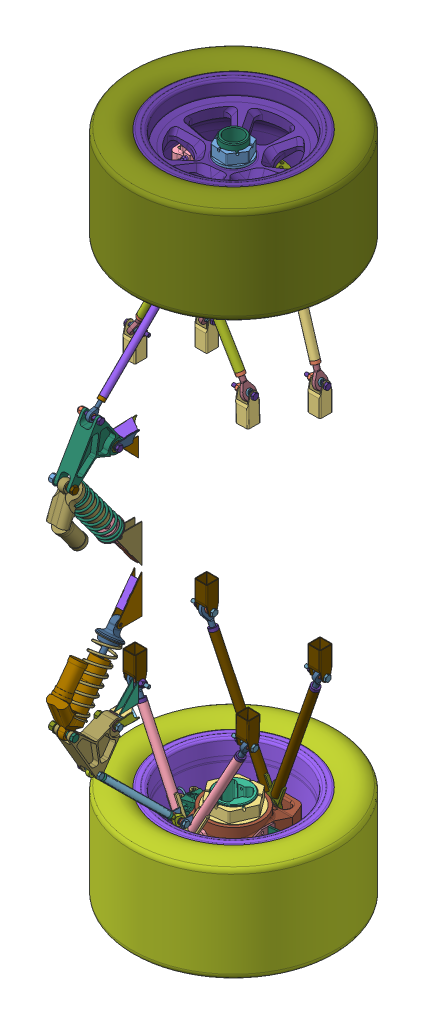
SolidWorks assembly UN-A1001-AA-Rear Unsprung Assembly, configuration Default. Lengths in mm.
Overall size (998.86 1363.58 600.2).
282 component instances, 120 part files, 8 mates.
Components (placement in the parent):
- SP-A0200-AH-Rear Axle Assembly-1: SP-A0200-AH-Rear Axle Assembly [Default] at origin size (935.94 549.59 593.34)
  - SP-AA-Rear Lower A-Arm^SP-A0200-AH-Rear Axle Assembly-1: SP-AA-Rear Lower A-Arm^SP-A0200-AH-Rear Axle Assembly [Default] at (0 -0.399 0.6588) x (1 0 0) z (0 0.002866 0.999996) size (222.76 290.57 36.42) (virtual)
    - SP-Lower Apex Rear-1: SP-Lower Apex Rear [Default] at (-792.4265 549.6462 121.5417) x (-0.932505 -0.360479 0.022123) z (0 -0.061256 -0.998122) size (54.94 63.8 9.53)
    - MirrorFS-MALE ROD END UNF-3A, 0.3125x24-0.25D (XAM-4)1-1: MirrorFS-MALE ROD END UNF-3A, 0.3125x24-0.25D (XAM-4)1 [Default] at (-906.7265 255.0788 139.6197) x (0.932505 -0.360479 0.022123) z (-0.361157 -0.930754 0.057121)
    - MirrorFS-MALE ROD END UNF-3A, 0.3125x24-0.25D (XAM-4)1-2: MirrorFS-MALE ROD END UNF-3A, 0.3125x24-0.25D (XAM-4)1 [Default] at (-678.1265 255.0788 139.6197) x (0.932505 0.360479 -0.022123) z (0.361157 -0.930754 0.057121)
    - SP-10003-AB-Threaded Insert-1: SP-10003-AB-Threaded Insert [A-Arm] at (-890.6731 296.4508 137.0806) x (0.932505 -0.360479 0.022123) z (-0.361157 -0.930754 0.057121) size (15.88 15.88 15.88)
    - SP-10003-AB-Threaded Insert-2: SP-10003-AB-Threaded Insert [A-Arm] at (-694.18 296.4508 137.0806) x (0.932505 0.360479 -0.022123) z (0.361157 -0.930754 0.057121) size (15.88 15.88 15.88)
    - SP-Rear Lower A-Arm Tube-1: SP-Rear Lower A-Arm Tube [Default] at (-838.6322 430.5677 128.8497) x (-0.361157 -0.930754 0.057121) z (0 -0.061256 -0.998122) size (257.84 15.88 15.88)
    - SP-Rear Lower A-Arm Tube-2: SP-Rear Lower A-Arm Tube [Default] at (-746.2209 430.5677 128.8497) x (0.361157 -0.930754 0.057121) z (0 0.061256 0.998122) size (257.84 15.88 15.88)
    - FS-HIGH MISALIGN SPHERICAL BEARING, 0.375-0.906D (3072-6G)-1: FS-HIGH MISALIGN SPHERICAL BEARING, 0.375-0.906D (3072-6G) [Default] at (-792.4265 549.6462 121.5417) x (-0.932505 0.360479 -0.022123) z (-0.361157 -0.930754 0.057121) size (26.46 21.71 26.13)
      - Race^FS-HIGH MISALIGN SPHERICAL BEARING, 0.375-0.906D (3072-6G)-1: Race^FS-HIGH MISALIGN SPHERICAL BEARING, 0.375-0.906D (3072-6G) [Default] at origin size (23.01 8.76 23.01) (virtual)
      - Ball^FS-HIGH MISALIGN SPHERICAL BEARING, 0.375-0.906D (3072-6G)-1: Ball^FS-HIGH MISALIGN SPHERICAL BEARING, 0.375-0.906D (3072-6G) [Default] x (0.359576 -0.008176 0.93308) z (-0.932238 -0.046516 0.358844) size (19.84 20.65 19.84) (virtual)
  - SP-AA-Rear Upper A-Arm^SP-A0200-AH-Rear Axle Assembly-1: SP-AA-Rear Upper A-Arm^SP-A0200-AH-Rear Axle Assembly [Default] at (-38.1 -1.9308 1.9372) x (1 0 0) z (0 0.00685 0.999977) size (216 215.55 29.43) (virtual)
    - SP-Upper Apex Rear-1: SP-Upper Apex Rear [Default] at (-755.8405 523.8827 293.8505) x (0.884705 -0.465567 -0.023329) z (0 -0.050046 0.998747) size (76.45 83.12 9.53)
    - MirrorFS-MALE ROD END UNF-3A, 0.3125x24-0.25D (XAM-4)1-1: MirrorFS-MALE ROD END UNF-3A, 0.3125x24-0.25D (XAM-4)1 [Default] at (-870.1405 307.2255 282.9942) x (0.884705 -0.465567 -0.023329) z (-0.466151 -0.883596 -0.044276)
    - MirrorFS-MALE ROD END UNF-3A, 0.3125x24-0.25D (XAM-4)1-2: MirrorFS-MALE ROD END UNF-3A, 0.3125x24-0.25D (XAM-4)1 [Default] at (-641.5405 307.2255 282.9942) x (0.884705 0.465567 0.023329) z (0.466151 -0.883596 -0.044276)
    - SP-10003-AB-Threaded Insert-1: SP-10003-AB-Threaded Insert [A-Arm] at (-849.4201 346.5014 284.9623) x (0.884705 -0.465567 -0.023329) z (-0.466151 -0.883596 -0.044276) size (15.88 15.88 15.88)
    - SP-10003-AB-Threaded Insert-2: SP-10003-AB-Threaded Insert [A-Arm] at (-662.261 346.5014 284.9623) x (0.884705 0.465567 0.023329) z (0.466151 -0.883596 -0.044276) size (15.88 15.88 15.88)
    - SP-Rear Upper A-Arm Tube-1: SP-Rear Upper A-Arm Tube [Default] at (-812.9905 415.5541 288.4224) x (0.466151 0.883596 0.044276) z (0.884705 -0.465567 -0.023329) size (186.28 15.88 15.88)
    - SP-Rear Upper A-Arm Tube-2: SP-Rear Upper A-Arm Tube [Default] at (-698.6905 415.5541 288.4224) x (-0.466151 0.883596 0.044276) z (0.884705 0.465567 0.023329) size (186.28 15.88 15.88)
    - FS-HIGH MISALIGN SPHERICAL BEARING, 0.375-0.906D (3072-6G)-1: FS-HIGH MISALIGN SPHERICAL BEARING, 0.375-0.906D (3072-6G) [Default] at (-755.8405 523.8827 293.8505) x (0.884705 -0.465567 -0.023329) z (-0.466151 -0.883596 -0.044276) size (26.46 21.71 26.13)
      - Race^FS-HIGH MISALIGN SPHERICAL BEARING, 0.375-0.906D (3072-6G)-1: Race^FS-HIGH MISALIGN SPHERICAL BEARING, 0.375-0.906D (3072-6G) [Default] at origin size (23.01 8.76 23.01) (virtual)
      - Ball^FS-HIGH MISALIGN SPHERICAL BEARING, 0.375-0.906D (3072-6G)-1: Ball^FS-HIGH MISALIGN SPHERICAL BEARING, 0.375-0.906D (3072-6G) [Default] x (0.359576 -0.008176 0.93308) z (-0.932238 -0.046516 0.358844) size (19.84 20.65 19.84) (virtual)
  - Assem8^SP-A0200-AH-Rear Axle Assembly-1: Assem8^SP-A0200-AH-Rear Axle Assembly [Default] at (-1592.9214 814.7933 712.2762) x (-0.999891 -0.01037 0.010464) z (0.012143 -0.982316 0.186836) size (17.98 166.51 230.13) (virtual)
    - Part2^Assem8_SP-A0200-AH-Rear Axle Assembly-1: Part2^Assem8_SP-A0200-AH-Rear Axle Assembly [Default] at origin size (15.39 113.92 157.78) (virtual)
    - SP-10003-AC-Threaded Insert-2: SP-10003-AC-Threaded Insert [AM-4 Rod End Thread] at (-799.064 427.6015 294.0449) x (-0.999891 -0.008342 0.012143) z (-0.014733 0.566176 -0.824153) size (12.7 12.7 15.88)
    - SP-10003-AC-Threaded Insert-3: SP-10003-AC-Threaded Insert [AM-4 Rod End Thread] at (-796.6527 334.9355 428.9338) x (-0.999891 -0.008342 0.012143) z (0.014733 -0.566176 0.824153) size (12.7 12.7 15.88)
    - FS-MALE ROD END UNF-3A, 0.25x28-0.25D (AM-4)-1: FS-MALE ROD END UNF-3A, 0.25x28-0.25D (AM-4) [Default] at (-796.0446 311.5665 462.9507) x (0 -0.824242 -0.566238) z (-0.014733 0.566176 -0.824153) size (19.32 14.06 49.44)
      - Body^FS-MALE ROD END UNF-3A, 0.25x28-0.25D (AM-4)-2: Body^FS-MALE ROD END UNF-3A, 0.25x28-0.25D (AM-4) [Default] at origin size (19.32 7.2 49.44) (virtual)
      - Ball^FS-MALE ROD END UNF-3A, 0.25x28-0.25D (AM-4)-2: Ball^FS-MALE ROD END UNF-3A, 0.25x28-0.25D (AM-4) [Default] x (0.09633 0.218783 0.971007) z (-0.984027 0.167661 0.059845) size (12.7 9.53 12.7) (virtual)
    - FS-MALE ROD END UNF-3A, 0.25x28-0.25D (AM-4)-2: FS-MALE ROD END UNF-3A, 0.25x28-0.25D (AM-4) [Default] at (-799.6721 450.9704 260.028) x (0 -0.824242 -0.566238) z (0.014733 -0.566176 0.824153) size (19.32 14.06 49.44)
      - Body^FS-MALE ROD END UNF-3A, 0.25x28-0.25D (AM-4)-2: Body^FS-MALE ROD END UNF-3A, 0.25x28-0.25D (AM-4) [Default] at origin size (19.32 7.2 49.44) (virtual)
      - Ball^FS-MALE ROD END UNF-3A, 0.25x28-0.25D (AM-4)-2: Ball^FS-MALE ROD END UNF-3A, 0.25x28-0.25D (AM-4) [Default] x (0.09633 0.218783 0.971007) z (-0.984027 0.167661 0.059845) size (12.7 9.53 12.7) (virtual)
  - SP-A0105-AC-Ohlin TTX25 MKII, 200mm-1: SP-A0105-AC-Ohlin TTX25 MKII, 200mm [Default] at (-793.9406 216.4917 537.8809) x (-1 0 0) z (0 0.803503 0.5953) size (48.39 85.02 197.6)
    - Shock Body^SP-A0105-AC-Ohlin TTX25 MKII, 200mm-1: Shock Body^SP-A0105-AC-Ohlin TTX25 MKII, 200mm [Default] at origin size (40.76 80 131.7) (virtual)
    - Head^SP-A0105-AC-Ohlin TTX25 MKII, 200mm-1: Head^SP-A0105-AC-Ohlin TTX25 MKII, 200mm [Default] at (0 0 -174.6) size (46 46 119) (virtual)
    - Ball^SP-A0105-AC-Ohlin TTX25 MKII, 200mm-1: Ball^SP-A0105-AC-Ohlin TTX25 MKII, 200mm [Default] at (0 0 -174.6) x (-0.011681 0.107343 0.994153) z (0.993776 0.111394 -0.000351) size (15 15 8) (virtual)
    - Ball^SP-A0105-AC-Ohlin TTX25 MKII, 200mm-2: Ball^SP-A0105-AC-Ohlin TTX25 MKII, 200mm [Default] x (0.079523 -0.862756 -0.499328) z (0.965926 -0.057074 0.252448) size (15 15 8) (virtual)
    - SP-#####-AB-Spring-1: SP-#####-AB-Spring [Default] at (0 0 -151.1) size (48.39 49.05 127.97)
  - FS-BALL BEARING, 0.25ID-0.75OD (60355K702)-1: FS-BALL BEARING, 0.25ID-0.75OD (60355K702) [Default] at (-784.8125 243.84 446.6415) x (0 -0.287121 0.957894) z (-1 0 0) size (19.05 19.05 7.14)
  - FS-BALL BEARING, 0.25ID-0.75OD (60355K702)-2: FS-BALL BEARING, 0.25ID-0.75OD (60355K702) [Default] at (-803.0688 243.84 446.6415) x (0 0.287121 -0.957894) z (1 0 0) size (19.05 19.05 7.14)
  - FS-CADMIUM PLATED C3 HEX, 0.25x28-1.65-0.469 (AN4-13A)-2: FS-CADMIUM PLATED C3 HEX, 0.25x28-1.65-0.469 (AN4-13A) [Default] at (-796.8362 310.0391 484.3789) x (-1 0 0) z (0 0.868755 0.495242) size (46.28 12.9 11.18)
  - FS-ZINC YELLOW CHROMATE C10.9 HX, M8x1.25-40-22 (95327A569)-1: FS-ZINC YELLOW CHROMATE C10.9 HX, M8x1.25-40-22 (95327A569) [Default] at (-795.4156 216.4917 537.8809) x (-1 0 0) z (0 -0.287121 0.957894) size (45.3 15.01 13)
  - FS-NYLOC FLHX C8, M8x1.25-11.1 (92461A400)-1: FS-NYLOC FLHX C8, M8x1.25-11.1 (92461A400) [Default] at (-820.9156 216.4917 537.8809) x (0 0.868058 -0.496463) z (-1 0 0) size (17.9 17.9 11.1)
  - FS-NYLOC G8 HX, 0.25x28-0.3125 (90630A145)-1: FS-NYLOC G8 HX, 0.25x28-0.3125 (90630A145) [Default] at (-809.8156 310.0391 484.3789) x (0 0.868058 -0.496463) z (0 0.496463 0.868058) size (11.11 7.94 12.83)
  - SP-C30066-AA-A-Arm Tab Box-1: SP-C30066-AA-A-Arm Tab Box [Default] at (-680.9758 289.7175 282.8202) x (-0.029021 0.999579 0) z (0 0 -1) size (60.32 25.4 25.4)
  - SP-C30066-AA-A-Arm Tab Box-2: SP-C30066-AA-A-Arm Tab Box [Default] at (-908.2405 289.7636 282.8202) x (0 1 0) z (0 0 -1) size (60.32 25.4 25.4)
  - SP-C30066-AA-A-Arm Tab Box-3: SP-C30066-AA-A-Arm Tab Box [Default] at (-678.1265 237.6164 139.5469) x (0 1 0) z (0 0 1) size (60.32 25.4 25.4)
  - SP-C30066-AA-A-Arm Tab Box-4: SP-C30066-AA-A-Arm Tab Box [Default] at (-906.7265 237.6164 139.5469) x (0 1 0) z (0 0 1) size (60.32 25.4 25.4)
  - MirrorSP-30063-AB-Pushrod Tab-1: MirrorSP-30063-AB-Pushrod Tab [Default] at (-782.0343 483.2134 293.6084) x (1 0 0) z (0 0.043203 -0.999066) size (1.59 15.88 23.81)
  - MirrorSP-30063-AB-Pushrod Tab-2: MirrorSP-30063-AB-Pushrod Tab [Default] at (-805.8468 483.2134 293.6084) x (-1 0 0) z (0 0.043203 -0.999066) size (1.59 15.88 23.81)
  - FS-NYLOC FLHX C8, M8x1.25-11.1 (92461A400)-2: FS-NYLOC FLHX C8, M8x1.25-11.1 (92461A400) [Default] at (-820.9156 243.84 446.6415) x (0 0 -1) z (-1 0 0) size (17.9 17.9 11.1)
  - FS-CADMIUM PLATED C3 HEX, 0.25x28-1.65-0.469 (AN4-13A)-3: FS-CADMIUM PLATED C3 HEX, 0.25x28-1.65-0.469 (AN4-13A) [Default] at (-796.8362 243.84 446.6415) x (-1 0 0) z (0 0.287121 -0.957894) size (46.28 12.9 11.18)
  - FS-CADMIUM PLATED C3 HEX, 0.25x28-1.65-0.469 (AN4-13A)-4: FS-CADMIUM PLATED C3 HEX, 0.25x28-1.65-0.469 (AN4-13A) [Default] at (-687.5506 306.9965 282.8202) x (-0.999579 -0.029021 0) z (0 0 -1) size (46.28 12.9 11.18)
  - FS-CADMIUM PLATED C3 HEX, 0.25x28-1.65-0.469 (AN4-13A)-5: FS-CADMIUM PLATED C3 HEX, 0.25x28-1.65-0.469 (AN4-13A) [Default] at (-902.1699 307.2261 282.8202) size (46.28 12.9 11.18)
  - FS-CADMIUM PLATED C3 HEX, 0.25x28-1.65-0.469 (AN4-13A)-6: FS-CADMIUM PLATED C3 HEX, 0.25x28-1.65-0.469 (AN4-13A) [Default] at (-912.7971 255.0789 139.5469) x (-1 0 0) z (0 0 -1) size (46.28 12.9 11.18)
  - FS-CADMIUM PLATED C3 HEX, 0.25x28-1.65-0.469 (AN4-13A)-7: FS-CADMIUM PLATED C3 HEX, 0.25x28-1.65-0.469 (AN4-13A) [Default] at (-684.1971 255.0789 139.5469) x (-1 0 0) z (0 0 -1) size (46.28 12.9 11.18)
  - FS-CADMIUM PLATED C3 HEX, 0.25x28-1.65-0.469 (AN4-13A)-8: FS-CADMIUM PLATED C3 HEX, 0.25x28-1.65-0.469 (AN4-13A) [Default] at (-799.2174 482.5275 309.4686) x (-1 0 0) z (0 -0.609051 0.793131) size (46.28 12.9 11.18)
  - FS-NYLOC G8 HX, 0.25x28-0.3125 (90630A145)-3: FS-NYLOC G8 HX, 0.25x28-0.3125 (90630A145) [Default] at (-807.4343 482.5275 309.4686) x (0 -0.043203 0.999066) z (0 -0.999066 -0.043203) size (11.11 7.94 12.83)
  - FS-NYLOC G8 HX, 0.25x28-0.3125 (90630A145)-4: FS-NYLOC G8 HX, 0.25x28-0.3125 (90630A145) [Default] at (-694.1772 306.8041 282.8202) x (-0.029021 0.999579 0) z (0 0 1) size (11.11 7.94 12.83)
  - FS-NYLOC G8 HX, 0.25x28-0.3125 (90630A145)-5: FS-NYLOC G8 HX, 0.25x28-0.3125 (90630A145) [Default] at (-895.5405 307.2261 282.8202) x (0 1 0) z (0 0 -1) size (11.11 7.94 12.83)
  - FS-NYLOC G8 HX, 0.25x28-0.3125 (90630A145)-6: FS-NYLOC G8 HX, 0.25x28-0.3125 (90630A145) [Default] at (-919.4265 255.0789 139.5469) x (0 1 0) z (0 0 1) size (11.11 7.94 12.83)
  - FS-NYLOC G8 HX, 0.25x28-0.3125 (90630A145)-7: FS-NYLOC G8 HX, 0.25x28-0.3125 (90630A145) [Default] at (-690.8265 255.0789 139.5469) x (0 -1 0) z (0 0 -1) size (11.11 7.94 12.83)
  - FS-ROD END RETAINING WASHER, 0.25-0.245 (NO PN)-5: FS-ROD END RETAINING WASHER, 0.25-0.245 (NO PN) [Default] at (-781.9073 482.5275 309.4686) x (0 1 0) z (-1 0 0) size (12.7 12.7 6.22)
  - FS-ROD END RETAINING WASHER, 0.25-0.245 (NO PN)-6: FS-ROD END RETAINING WASHER, 0.25-0.245 (NO PN) [Default] at (-805.9738 482.5275 309.4686) x (0 0.978954 0.204082) z (1 0 0) size (12.7 12.7 6.22)
  - SP-A0200-Rear Inner Rocker Gusset-1: SP-A0200-Rear Inner Rocker Gusset [Default] at (-793.9406 234.6955 425.4808) x (1 0 0) z (0 0.052336 0.99863) size (26.99 1.59 48.67)
  - SP-A0200-Rear Long Rocker Tab-1: SP-A0200-Rear Long Rocker Tab [Rear] at (-807.4344 243.84 446.6415) x (1 0 0) z (0 -0.00621 -0.999981) size (1.59 19.05 73.11)
  - SP-A0200-Rear Outer Rocker Gusset-1: SP-A0200-Rear Outer Rocker Gusset [Default] at (-793.9406 251.3902 418.9606) x (1 0 0) z (0 -0.039929 0.999203) size (26.99 1.59 43.52)
  - SP-A0200-Rear Rocker Gusset Support-1: SP-A0200-Rear Rocker Gusset Support [Default] at (-800.2906 228.5949 403.7833) x (0 0 1) z (0 1 0) size (38.05 1.59 40.09)
  - SP-A0200-Rear Short Rocker Tab-1: SP-A0200-Rear Short Rocker Tab [Rear] at (-780.4469 243.8408 446.6212) x (1 0 0) z (0 -0.00621 -0.999981) size (1.59 17.17 50.59)
  - SP-A0200-Rear Rocker Gusset Support-2: SP-A0200-Rear Rocker Gusset Support [Default] at (-789.8131 228.5949 403.7833) x (0 0 1) z (0 1 0) size (38.05 1.59 40.09)
  - SP-A0200-Rear Shock Gusset-1: SP-A0200-Rear Shock Gusset [Default] at (-793.9406 34.3591 413.4634) x (1 0 0) z (0 0.809017 0.587785) size (14.29 1.59 50.8)
  - SP-A0200-Rear Shock Tab-1: SP-A0200-Rear Shock Tab [Rear] at (-786.7969 76.2 433.9415) x (-1 0 0) z (0 -0.809017 -0.587785) size (1.59 45.95 88.76)
  - SP-A0200-Rear Shock Tab-2: SP-A0200-Rear Shock Tab [Front] at (-801.0844 76.2 433.9415) x (-1 0 0) z (0 -0.809017 -0.587785) size (1.59 45.95 88.76)
  - FS-MALE ROD END UNJF-3A, 0.375x24-0.25D (HXAM-4T)-4: FS-MALE ROD END UNJF-3A, 0.375x24-0.25D (HXAM-4T) [Simplified] at (-679.6405 307.2261 282.8202) x (0 0.043203 -0.999066) z (-0.466151 0.883879 0.038222) size (26.22 15.06 62.54)
    - Body^FS-MALE ROD END UNJF-3A, 0.375x24-0.25D (HXAM-4T)-1: Body^FS-MALE ROD END UNJF-3A, 0.375x24-0.25D (HXAM-4T) [no_threads] at origin size (26.22 9.62 62.54)
    - Ball^FS-MALE ROD END UNJF-3A, 0.375x24-0.25D (HXAM-4T)-1: Ball^FS-MALE ROD END UNJF-3A, 0.375x24-0.25D (HXAM-4T) [Default] at origin size (15.06 15.06 15.06)
  - FS-MALE ROD END UNJF-3A, 0.375x24-0.25D (HXAM-4T)-5: FS-MALE ROD END UNJF-3A, 0.375x24-0.25D (HXAM-4T) [Simplified] at (-908.2405 307.2261 282.8202) x (0 -0.043203 0.999066) z (0.466151 0.883879 0.038222) size (26.22 15.06 62.54)
    - Body^FS-MALE ROD END UNJF-3A, 0.375x24-0.25D (HXAM-4T)-1: Body^FS-MALE ROD END UNJF-3A, 0.375x24-0.25D (HXAM-4T) [no_threads] at origin size (26.22 9.62 62.54)
    - Ball^FS-MALE ROD END UNJF-3A, 0.375x24-0.25D (HXAM-4T)-1: Ball^FS-MALE ROD END UNJF-3A, 0.375x24-0.25D (HXAM-4T) [Default] at origin size (15.06 15.06 15.06)
  - FS-MALE ROD END UNJF-3A, 0.375x24-0.25D (HXAM-4T)-6: FS-MALE ROD END UNJF-3A, 0.375x24-0.25D (HXAM-4T) [Simplified] at (-906.7265 255.0789 139.5469) x (0 0.064116 0.997942) z (0.361157 0.930586 -0.059789) size (26.22 15.06 62.54)
    - Body^FS-MALE ROD END UNJF-3A, 0.375x24-0.25D (HXAM-4T)-1: Body^FS-MALE ROD END UNJF-3A, 0.375x24-0.25D (HXAM-4T) [no_threads] at origin size (26.22 9.62 62.54)
    - Ball^FS-MALE ROD END UNJF-3A, 0.375x24-0.25D (HXAM-4T)-1: Ball^FS-MALE ROD END UNJF-3A, 0.375x24-0.25D (HXAM-4T) [Default] at origin size (15.06 15.06 15.06)
  - FS-MALE ROD END UNJF-3A, 0.375x24-0.25D (HXAM-4T)-7: FS-MALE ROD END UNJF-3A, 0.375x24-0.25D (HXAM-4T) [Simplified] at (-678.1265 255.0789 139.5469) x (0 -0.064116 -0.997942) z (-0.361157 0.930586 -0.059789) size (26.22 15.06 62.54)
    - Body^FS-MALE ROD END UNJF-3A, 0.375x24-0.25D (HXAM-4T)-1: Body^FS-MALE ROD END UNJF-3A, 0.375x24-0.25D (HXAM-4T) [no_threads] at origin size (26.22 9.62 62.54)
    - Ball^FS-MALE ROD END UNJF-3A, 0.375x24-0.25D (HXAM-4T)-1: Ball^FS-MALE ROD END UNJF-3A, 0.375x24-0.25D (HXAM-4T) [Default] at origin size (15.06 15.06 15.06)
  - SP-B0100-Rear Rocker-1: SP-B0100-Rear Rocker [Default] at (14.7593 458.8134 -310.4211) x (0.993764 -0.111506 -0.000215) z (-0.085107 -0.759728 0.644647) size (43.51 92.41 122.03)
- WT-A0100-XG-Corner Assembly-1: WT-A0100-XG-Corner Assembly [Front Left Corner Assembly] at origin size (260.47 172.81 260.47)
  - WT-00202-AA-Hoosier R25B 16x7_5-10-1: WT-00202-AA-Hoosier R25B 16x7_5-10 [Default] at (-793.1174 574.9879 198.909) x (-1 0 0) z (0 -1 0.000253) size (411.48 411.48 213.5)
  - WT-00201-AA-OZ Centerlock 10in Wheel-1: WT-00201-AA-OZ Centerlock 10in Wheel [Default] at (-793.1174 596.9879 198.9034) x (-0.992442 0.000031 0.122714) z (0 1 -0.000253) size (288.79 288.79 189.86)
  - WT-10105-AA-Drive Pin-8: WT-10105-AA-Drive Pin [Default] at (-825.0424 596.994 223.0032) x (-0.121576 0.000251 0.992582) z (-0.992582 -0.000031 -0.121576) size (12.67 23.01 11.95)
  - WT-10102-AA-Centerlock Nut-1: WT-10102-AA-Centerlock Nut [Default] at (-793.1174 647.6073 198.8906) x (-0.440541 -0.000227 -0.897732) z (0.897733 -0.000111 -0.440541) size (66 31.75 66)
  - WT-XF-Upright-1: WT-XF-Upright [Default] at (-793.1174 537.8923 198.9183) x (-0.999961 -0.000002 -0.008824) z (-0.008824 0.000253 0.999961) size (134.42 50.23 211.08)
  - BR-A0102-AA-Caliper Assembly-1: BR-A0102-AA-Caliper Assembly [Default] at (-874.0145 570.8565 194.5235) x (-0.069854 0.000252 0.997557) z (0 -1 0.000253) size (40.11 43.54 52.73)
    - cp3838-M08x1.25m_CP4477-110^BR-A0102-AA-Caliper Assembly-1: cp3838-M08x1.25m_CP4477-110^BR-A0102-AA-Caliper Assembly [Default] at (-13.37 19.3 19.55) x (-0.999952 -0.009843 0) z (0 0 -1) size (13 13 46) (virtual)
    - CP4226-102^BR-A0102-AA-Caliper Assembly-1: CP4226-102^BR-A0102-AA-Caliper Assembly [Default] x (-1 0 0) z (0 0 -1) size (63.87 47.42 31.57) (virtual)
    - cp4226-104_CP4226-104^BR-A0102-AA-Caliper Assembly-1: cp4226-104_CP4226-104^BR-A0102-AA-Caliper Assembly [Default] at (0 23 -31.9644) x (0 0 1) z (-1 0 0) size (61.35 20.1 3) (virtual)
    - CP4226-101^BR-A0102-AA-Caliper Assembly-1: CP4226-101^BR-A0102-AA-Caliper Assembly [Default] at origin size (81.26 55.69 34.68) (virtual)
    - cp3838-M08x1.25m_CP4477-110^BR-A0102-AA-Caliper Assembly-2: cp3838-M08x1.25m_CP4477-110^BR-A0102-AA-Caliper Assembly [Default] at (13.37 19.3 19.55) x (-0.997666 -0.068288 0) z (0 0 -1) size (13 13 46) (virtual)
    - cp3049-40a_CP4226-103^BR-A0102-AA-Caliper Assembly-1: cp3049-40a_CP4226-103^BR-A0102-AA-Caliper Assembly [Default] at (0 0 10.305) x (-0.993137 0.116957 0) z (0 0 -1) size (25.2 25.2 14.87) (virtual)
    - CP4469-101^BR-A0102-AA-Caliper Assembly-1: CP4469-101^BR-A0102-AA-Caliper Assembly [Default] at (42 -11.5 -23.98) x (0 -0.520643 0.853775) z (-1 0 0) size (9.18 8.2 29.15) (virtual)
    - cp3049-40a_CP4226-103^BR-A0102-AA-Caliper Assembly-2: cp3049-40a_CP4226-103^BR-A0102-AA-Caliper Assembly [Default] at (0 0 -10.305) size (25.2 25.2 14.87) (virtual)
    - Brake Pad^BR-A0102-AA-Caliper Assembly-1: Brake Pad^BR-A0102-AA-Caliper Assembly [Default] at (0 11.1798 8.5855) x (-1 0 0) z (0 -1 0) size (39.62 6.86 43.54) (virtual)
    - Brake Pad^BR-A0102-AA-Caliper Assembly-2: Brake Pad^BR-A0102-AA-Caliper Assembly [Default] at (0 11.1798 -8.5905) x (1 0 0) z (0 -1 0) size (39.62 6.86 43.54) (virtual)
  - WT-10103-AA-Grease Seal-1: WT-10103-AA-Grease Seal [Default] at (-793.1174 559.091 198.913) x (-0.781145 -0.000158 -0.624349) z (-0.624349 0.000198 0.781145) size (97.66 13.92 97.66)
  - LL713049-LL713010-TheTimkenCompany-3D-11-03-2022.stp-1: LL713049-LL713010-TheTimkenCompany-3D-11-03-2022.stp [Default] at (-793.1174 541.0673 198.9175) x (0 1 -0.000253) z (0.586717 -0.000205 -0.809792) size (15.53 98.42 98.42)
  - LL713049-LL713010-TheTimkenCompany-3D-11-03-2022.stp-2: LL713049-LL713010-TheTimkenCompany-3D-11-03-2022.stp [Default] at (-793.1174 534.7173 198.9191) x (0 -1 0.000253) z (0.531557 -0.000214 -0.847022) size (15.53 98.42 98.42)
  - WT-XA-Tripod Nut-1: WT-XA-Tripod Nut [Default] at (-793.1174 516.4598 198.9238) x (0 1 -0.000253) z (0.798123 -0.000152 -0.602494) size (30.44 98.37 98.37)
  - WT-BA-Camber Block-1: WT-BA-Camber Block [Default] at (-793.95 547.3609 293.2547) x (-0.999961 -0.000002 -0.008824) z (-0.008819 -0.034647 0.999361) size (82.61 35.93 35.38)
  - 91290A442_Alloy Steel Socket Head Screw-1: 91290A442_Alloy Steel Socket Head Screw [91290A442] at (-816.177 556.8302 293.3869) x (0.914102 0.014329 -0.405231) z (0.000308 -0.9994 -0.034645) size (13 13 48.09)
  - BR-A0000-AB-Rear Brake Assembly-1: BR-A0000-AB-Rear Brake Assembly [Default No Bobbins] at (-793.1174 596.9879 198.9034) x (-0.602494 -0.000202 -0.798123) z (-0.798123 0.000152 0.602494) size (251.55 172.72 251.55)
    - WT-XA-#####-Tripod Hub-2: WT-XA-#####-Tripod Hub [Default] at origin size (102.86 172.72 102.86)
    - BR-20601-AB-Brake Rotor-1: BR-20601-AB-Brake Rotor [Default] at (0 26.1303 0) x (0.866025 0 -0.5) z (0.5 0 0.866025) size (184.15 4.76 184.15)
    - BR-20603-BA-Floating Bobbins-1: BR-20603-BA-Floating Bobbins [Default] at (39.8696 25.9874 23.0188) size (15.88 8.92 15.88)
    - BR-20603-BA-Floating Bobbins-2: BR-20603-BA-Floating Bobbins [Default] at (0 25.9874 46.0375) x (0.5 0 0.866025) z (-0.866025 0 0.5) size (15.88 8.92 15.88)
    - BR-20603-BA-Floating Bobbins-3: BR-20603-BA-Floating Bobbins [Default] at (-39.8696 25.9874 23.0188) x (-0.5 0 0.866025) z (-0.866025 0 -0.5) size (15.88 8.92 15.88)
    - BR-20603-BA-Floating Bobbins-4: BR-20603-BA-Floating Bobbins [Default] at (-39.8696 25.9874 -23.0188) x (-1 0 0) z (0 0 -1) size (15.88 8.92 15.88)
    - BR-20603-BA-Floating Bobbins-5: BR-20603-BA-Floating Bobbins [Default] at (0 25.9874 -46.0375) x (-0.5 0 -0.866025) z (0.866025 0 -0.5) size (15.88 8.92 15.88)
    - BR-20603-BA-Floating Bobbins-6: BR-20603-BA-Floating Bobbins [Default] at (39.8696 25.9874 -23.0188) x (0.5 0 -0.866025) z (0.866025 0 0.5) size (15.88 8.92 15.88)
    - WT-20104-AB-Rear Sensor Ring-1: WT-20104-AB-Rear Sensor Ring [Default] at (0 30.099 0) x (0.882948 0 -0.469472) z (0 -1 0) size (137 137 1.59)
    - 91590A121_External Retaining Ring-1: 91590A121_External Retaining Ring [91590A121] at (-39.8696 29.2354 23.0188) x (0 1 0) z (-0.857167 0 0.515038) size (0.64 14.63 13.25)
    - 91590A121_External Retaining Ring-2: 91590A121_External Retaining Ring [91590A121] at (-39.8696 29.2354 -23.0188) x (0 1 0) z (-0.87462 0 -0.48481) size (0.64 14.63 13.25)
    - 91590A121_External Retaining Ring-3: 91590A121_External Retaining Ring [91590A121] at (0 29.2354 -46.0375) x (0 1 0) z (-0.017452 0 -0.999848) size (0.64 14.63 13.25)
    - 91590A121_External Retaining Ring-4: 91590A121_External Retaining Ring [91590A121] at (39.8696 29.2354 -23.0188) x (0 1 0) z (0.857167 0 -0.515038) size (0.64 14.63 13.25)
    - 91590A121_External Retaining Ring-5: 91590A121_External Retaining Ring [91590A121] at (39.8696 29.2354 23.0188) x (0 1 0) z (0.87462 0 0.48481) size (0.64 14.63 13.25)
    - 91590A121_External Retaining Ring-6: 91590A121_External Retaining Ring [91590A121] at (0 29.2354 46.0375) x (0 1 0) z (0.017452 0 0.999848) size (0.64 14.63 13.25)
    - 97447A110_Aluminum Blind Rivets with Aluminum Mandrel-1: 97447A110_Aluminum Blind Rivets with Aluminum Mandrel [97447A110] at (9.6137 30.099 51.8707) x (-0.302097 0 -0.953277) z (0 1 0) size (5.03 5.03 11.56)
    - 97447A110_Aluminum Blind Rivets with Aluminum Mandrel-2: 97447A110_Aluminum Blind Rivets with Aluminum Mandrel [97447A110] at (-40.1145 30.099 34.261) x (0.674514 0 -0.738262) z (0 1 0) size (5.03 5.03 11.56)
    - 97447A110_Aluminum Blind Rivets with Aluminum Mandrel-3: 97447A110_Aluminum Blind Rivets with Aluminum Mandrel [97447A110] at (-49.7282 30.099 -17.6097) x (0.976611 0 0.215015) z (0 1 0) size (5.03 5.03 11.56)
    - 97447A110_Aluminum Blind Rivets with Aluminum Mandrel-4: 97447A110_Aluminum Blind Rivets with Aluminum Mandrel [97447A110] at (-9.6137 30.099 -51.8707) x (0.302097 0 0.953277) z (0 1 0) size (5.03 5.03 11.56)
    - 97447A110_Aluminum Blind Rivets with Aluminum Mandrel-5: 97447A110_Aluminum Blind Rivets with Aluminum Mandrel [97447A110] at (40.1145 30.099 -34.261) x (-0.674514 0 0.738262) z (0 1 0) size (5.03 5.03 11.56)
    - 97447A110_Aluminum Blind Rivets with Aluminum Mandrel-6: 97447A110_Aluminum Blind Rivets with Aluminum Mandrel [97447A110] at (49.7282 30.099 17.6097) x (-0.976611 0 -0.215015) z (0 1 0) size (5.03 5.03 11.56)
  - FS-Jet Nut, M8x1.25 (MJET-M8X1.25)-1: FS-Jet Nut, M8x1.25 (MJET-M8X1.25) [Default] at (-816.1783 561.0546 293.5333) x (-0.906747 0.01433 -0.421432) z (-0.000308 0.9994 0.034645) size (13.6 13.6 7)
  - 91290A442_Alloy Steel Socket Head Screw-2: 91290A442_Alloy Steel Socket Head Screw [91290A442] at (-771.7287 556.8303 293.7791) x (-0.549228 0.028783 -0.835176) z (0.000308 -0.9994 -0.034645) size (13 13 48.09)
  - FS-Jet Nut, M8x1.25 (MJET-M8X1.25)-2: FS-Jet Nut, M8x1.25 (MJET-M8X1.25) [Default] at (-771.73 561.0547 293.9256) x (0.139109 0.034351 -0.989681) z (-0.000308 0.9994 0.034645) size (13.6 13.6 7)
  - WT-10105-AA-Drive Pin-21: WT-10105-AA-Drive Pin [Default] at (-769.0177 596.9959 230.8283) x (0.992582 0.000031 0.121576) z (-0.121576 0.000251 0.992582) size (12.67 23.01 11.95)
  - WT-10105-AA-Drive Pin-22: WT-10105-AA-Drive Pin [Default] at (-761.1925 596.9818 174.8036) x (0.121576 -0.000251 -0.992582) z (0.992582 0.000031 0.121576) size (12.67 23.01 11.95)
  - WT-10105-AA-Drive Pin-23: WT-10105-AA-Drive Pin [Default] at (-817.2172 596.9798 166.9785) x (-0.992582 -0.000031 -0.121576) z (0.121576 -0.000251 -0.992582) size (12.67 23.01 11.95)
  - WT-AA-#####-Rear Toe Backing Plate-1: WT-AA-#####-Rear Toe Backing Plate [Default] at (-737.6079 537.8924 199.4082) x (0.999961 0.000002 0.008824) z (-0.008824 0.000253 0.999961) size (3.17 25.4 50.8)
  - WT-AA-#####-Rear Toe Top Clevis-1: WT-AA-#####-Rear Toe Top Clevis [Default] at (-737.7085 541.0703 210.8115) x (0.999961 0.000002 0.008824) z (-0.008824 0.000253 0.999961) size (31.75 27.83 3.17)
  - WT-AA-#####-Rear Toe Bottom Clevis-1: WT-AA-#####-Rear Toe Bottom Clevis [Default] at (-737.4815 537.8888 185.0832) x (0.999961 0.000002 0.008824) z (-0.008824 0.000253 0.999961) size (31.75 27.12 3.17)
- MirrorWT-A0100-XG-Corner Assembly-2: MirrorWT-A0100-XG-Corner Assembly [Default] x (1 0 0) z (0 0 -1) size (411.48 213.6 411.53)
  - MirrorWT-00202-AA-Hoosier R25B 16x7_5-10-1: MirrorWT-00202-AA-Hoosier R25B 16x7_5-10 [Default] at (-793.1174 574.9879 -198.909) x (-1 0 0) z (0 1 0.000253) size (411.48 411.48 213.5)
  - MirrorWT-00201-AA-OZ Centerlock 10in Wheel-1: MirrorWT-00201-AA-OZ Centerlock 10in Wheel [Default] at (-793.1174 596.9879 -198.9034) x (-0.992442 0.000031 -0.122714) z (0 -1 -0.000253) size (288.79 288.79 189.86)
  - MirrorWT-10105-AA-Drive Pin-1: MirrorWT-10105-AA-Drive Pin [Default] at (-825.0424 596.994 -223.0032) x (-0.121576 0.000251 -0.992582) z (0.992582 0.000031 -0.121576) size (12.67 23.01 11.95)
  - MirrorWT-10102-AA-Centerlock Nut-1: MirrorWT-10102-AA-Centerlock Nut [Default] at (-793.1174 647.6073 -198.8906) x (-0.440541 -0.000227 0.897732) z (-0.897733 0.000111 -0.440541) size (66 31.75 66)
  - MirrorWT-XF-Upright-1: MirrorWT-XF-Upright [Default] at (-793.1174 537.8923 -198.9183) x (-0.999961 -0.000002 0.008824) z (0.008824 -0.000253 0.999961) size (134.42 50.23 211.08)
  - MirrorBR-A0102-AA-Caliper Assembly-1: MirrorBR-A0102-AA-Caliper Assembly [Default] at (-874.0145 570.8565 -194.5235) x (-0.069854 0.000252 -0.997557) z (0 1 0.000253) size (82.63 68.94 66.64)
    - Mirrorcp3838-M08x1.25m_CP4477-110^MirrorBR-A0102-AA-Caliper Assembly-1: Mirrorcp3838-M08x1.25m_CP4477-110^BR-A0102-AA-Caliper Assembly [Default] at (-13.37 19.3 -19.55) x (-0.999952 -0.009843 0) z (0 0 -1) size (13 13 46) (virtual)
    - MirrorCP4226-102^MirrorBR-A0102-AA-Caliper Assembly-1: MirrorCP4226-102^BR-A0102-AA-Caliper Assembly [Default] x (-1 0 0) z (0 0 -1) size (63.87 47.42 31.57) (virtual)
    - Mirrorcp4226-104_CP4226-104^MirrorBR-A0102-AA-Caliper Assembly-1: Mirrorcp4226-104_CP4226-104^BR-A0102-AA-Caliper Assembly [Default] at (0 23 31.9644) x (0 0 -1) z (1 0 0) size (61.35 20.1 3) (virtual)
    - MirrorCP4226-101^MirrorBR-A0102-AA-Caliper Assembly-1: MirrorCP4226-101^BR-A0102-AA-Caliper Assembly [Default] at origin size (81.26 55.69 34.68) (virtual)
    - Mirrorcp3838-M08x1.25m_CP4477-110^MirrorBR-A0102-AA-Caliper Assembly-2: Mirrorcp3838-M08x1.25m_CP4477-110^BR-A0102-AA-Caliper Assembly [Default] at (13.37 19.3 -19.55) x (-0.997666 -0.068288 0) z (0 0 -1) size (13 13 46) (virtual)
    - Mirrorcp3049-40a_CP4226-103^MirrorBR-A0102-AA-Caliper Assembly-1: Mirrorcp3049-40a_CP4226-103^BR-A0102-AA-Caliper Assembly [Default] at (0 0 -10.305) x (-0.993137 0.116957 0) z (0 0 -1) size (25.2 25.2 14.87) (virtual)
    - MirrorCP4469-101^MirrorBR-A0102-AA-Caliper Assembly-1: MirrorCP4469-101^BR-A0102-AA-Caliper Assembly [Default] at (42 -11.5 23.98) x (0 -0.520643 -0.853775) z (1 0 0) size (9.18 8.2 29.15) (virtual)
    - Mirrorcp3049-40a_CP4226-103^MirrorBR-A0102-AA-Caliper Assembly-2: Mirrorcp3049-40a_CP4226-103^BR-A0102-AA-Caliper Assembly [Default] at (0 0 10.305) size (25.2 25.2 14.87) (virtual)
    - MirrorBrake Pad^MirrorBR-A0102-AA-Caliper Assembly-1: MirrorBrake Pad^BR-A0102-AA-Caliper Assembly [Default] at (0 11.1798 -8.5855) x (-1 0 0) z (0 1 0) size (39.62 6.86 43.54) (virtual)
    - MirrorBrake Pad^MirrorBR-A0102-AA-Caliper Assembly-2: MirrorBrake Pad^BR-A0102-AA-Caliper Assembly [Default] at (0 11.1798 8.5905) x (1 0 0) z (0 1 0) size (39.62 6.86 43.54) (virtual)
  - MirrorWT-10103-AA-Grease Seal-1: MirrorWT-10103-AA-Grease Seal [Default] at (-793.1174 559.091 -198.913) x (-0.781145 -0.000158 0.624349) z (0.624349 -0.000198 0.781145) size (97.66 13.92 97.66)
  - MirrorLL713049-LL713010-TheTimkenCompany-3D-11-03-2022.stp-1: MirrorLL713049-LL713010-TheTimkenCompany-3D-11-03-2022.stp [Default] at (-793.1174 541.0673 -198.9175) x (0 1 0.000253) z (-0.586717 0.000205 -0.809792) size (15.53 98.42 98.42)
  - MirrorLL713049-LL713010-TheTimkenCompany-3D-11-03-2022.stp-2: MirrorLL713049-LL713010-TheTimkenCompany-3D-11-03-2022.stp [Default] at (-793.1174 534.7173 -198.9191) x (0 -1 -0.000253) z (-0.531557 0.000214 -0.847022) size (15.53 98.42 98.42)
  - MirrorWT-XA-Tripod Nut-1: MirrorWT-XA-Tripod Nut [Default] at (-793.1174 516.4598 -198.9238) x (0 1 0.000253) z (-0.798123 0.000152 -0.602494) size (30.44 98.37 98.37)
  - MirrorWT-BA-Camber Block-1: MirrorWT-BA-Camber Block [Default] at (-793.95 547.3609 -293.2547) x (-0.999961 -0.000002 0.008824) z (0.008819 0.034647 0.999361) size (82.61 35.93 35.38)
  - Mirror91290A442_Alloy Steel Socket Head Screw-1: Mirror91290A442_Alloy Steel Socket Head Screw [91290A442] at (-816.177 556.8302 -293.3869) x (0.914102 0.014329 0.405231) z (-0.000308 0.9994 -0.034645) size (13 13 48.09)
  - MirrorBR-A0000-AB-Rear Brake Assembly-1: MirrorBR-A0000-AB-Rear Brake Assembly [Default] at (-793.1174 596.9879 -198.9034) x (-0.602494 -0.000202 0.798123) z (0.798123 -0.000152 0.602494) size (251.55 172.72 251.55)
    - MirrorWT-XA-#####-Tripod Hub-1: MirrorWT-XA-#####-Tripod Hub [Default] at origin size (102.86 172.72 102.86)
    - MirrorBR-20601-AB-Brake Rotor-1: MirrorBR-20601-AB-Brake Rotor [Default] at (0 26.1303 0) x (0.866025 0 0.5) z (-0.5 0 0.866025) size (184.15 4.76 184.15)
    - MirrorBR-20603-BA-Floating Bobbins-1: MirrorBR-20603-BA-Floating Bobbins [Default] at (39.8696 25.9874 -23.0188) size (15.88 8.92 15.88)
    - MirrorBR-20603-BA-Floating Bobbins-2: MirrorBR-20603-BA-Floating Bobbins [Default] at (0 25.9874 -46.0375) x (0.5 0 -0.866025) z (0.866025 0 0.5) size (15.88 8.92 15.88)
    - MirrorBR-20603-BA-Floating Bobbins-3: MirrorBR-20603-BA-Floating Bobbins [Default] at (-39.8696 25.9874 -23.0188) x (-0.5 0 -0.866025) z (0.866025 0 -0.5) size (15.88 8.92 15.88)
